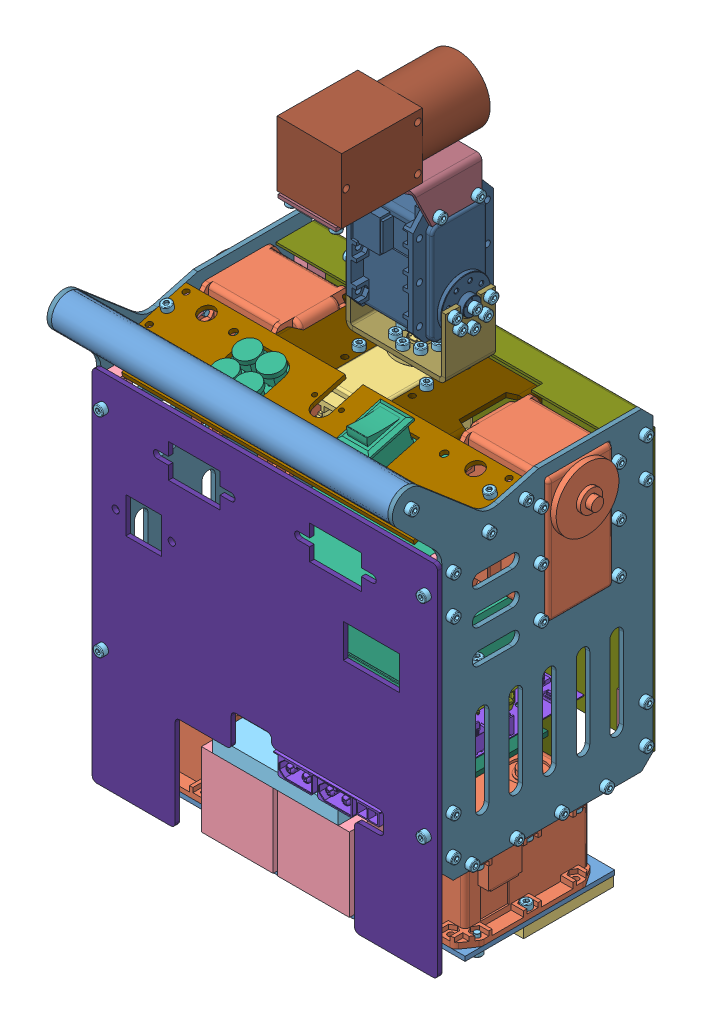
SolidWorks assembly 躯干, configuration 默认. Lengths in mm.
Overall size (172 287.24 163.85).
149 component instances, 24 part files, 310 mates.
Components (placement in the parent):
- 机器人-下腰骨-1: 机器人-下腰骨 [默认] at (14.1339 4.9855 143.3) size (150 2 94.2)
- 机器人-腰部连接件-1: 机器人-腰部连接件 [默认] at (86.3339 40.9855 146.55) size (5.6 6 68)
- 机器人-腰部连接件-2: 机器人-腰部连接件 [默认] at (-58.0661 40.9855 146.55) size (5.6 6 68)
- 机器人-腰部支撑件-1: 机器人-腰部支撑件 [默认] at (69.0339 0.6855 128.55) x (0 0 -1) z (1 0 0) size (40 4.3 40.2)
- 机器人-腰部支撑件-2: 机器人-腰部支撑件 [默认] at (-40.7661 0.6855 128.55) x (0 0 -1) z (1 0 0) size (40 4.3 40.2)
- 电池组-1: 电池组 [默认] at (-73.6661 8.3922 158.5613) x (0 -1 0) z (1 0 0) size (40 92 66)
  - 大电池-1: 大电池 [默认] at (-15.0933 -28.8887 72) size (33 78 32)
  - 大电池-2: 大电池 [默认] at (-15.0933 -28.8887 106) size (33 78 32)
  - 小电池-1: 小电池 [默认] at (-35.0933 63.1113 89) x (0 0 1) z (0 -1 0) size (56 7 92)
- 电路-1: 电路 [默认] at (-149.9254 121.6563 46.2423) x (0.629094 0.186421 -0.754644) z (0.775792 -0.211602 0.594451) size (135.66 81.1 136.29)
  - TX2-1: TX2 [默认] at (66.6739 -13.371 209.1651) x (-0.629094 -0.048866 -0.775792) z (0.186421 0.959412 -0.211602) size (87.07 50.04 32.13)
  - 9003-1: 9003 [默认] at (15.6894 -27.7493 144.427) x (0.629094 0.048866 0.775792) z (-0.186421 -0.959412 0.211602) size (96.22 72.67 50.58)
  - Main-1: Main [默认] at (20.5563 -29.3993 193.2183) x (0.629094 0.048866 0.775792) z (0.186421 0.959412 -0.211602) size (100 91.07 21.61)
- 机器人-背板-1: 机器人-背板 [默认] at (14.1339 173.2258 167.0875) x (1 0 0) z (0 -0.258819 0.965926) size (150 2 40)
- 脑袋-1: 脑袋 [默认] at (31.3694 207.3211 170.3695) x (-0.999965 0 -0.008321) z (0.008321 0 -0.999965) size (45.6 104.22 67.8)
  - MX28-2-1: MX28-2 [默认] at (67.0789 12.1977 37.204) x (0 0 -1) z (-1 0 0) size (35.6 50.71 44.45)
  - 工业摄像头-1: 工业摄像头 [默认] at (17.9784 61.4039 35.5741) x (-1 0 0) z (0 1 0) size (29 65.7 29)
  - 机器人-脖子-1: 机器人-脖子 [默认] at (17.6701 -26.3128 48.8741) size (106 27.37 22)
  - 机器人-摄像头固定件-1: 机器人-摄像头固定件 [默认] at (17.9784 46.9039 59.8741) x (-1 0 0) z (0 1 0) size (62.95 61 17.05)
- 机器人-侧板-3: 机器人-侧板 [默认] at (-60.8661 139.1722 141.05) x (0 0 1) z (-1 0 0) size (116.15 161.21 2)
- 机器人-侧板-4: 机器人-侧板 [默认] at (91.1339 139.1722 141.05) x (0 0 1) z (-1 0 0) size (116.15 161.21 2)
- 机器人-上腰骨-2: 机器人-上腰骨 [默认] at (14.1339 48.9855 149.05) size (100.8 2 61)
- 机器人-前盖-2: 机器人-前盖 [默认] at (14.1339 110.9855 94.95) x (1 0 0) z (0 -1 0) size (154 19.53 171.5)
- 机器人-后盖-2: 机器人-后盖 [默认] at (14.1339 100.9855 188.95) size (154 160 2)
- 机器人-肩骨-1: 机器人-肩骨 [默认] at (-24.8661 182.5355 128.55) size (28.68 11.38 40.2)
- 机器人-肩骨-2: 机器人-肩骨 [默认] at (53.1339 182.5355 128.55) x (-1 0 0) z (0 0 -1) size (28.68 11.38 40.2)
- 提手-1: 提手 [默认] at (-60.8661 194.6934 203.5985) size (150 15 15)
- MX64-1: MX64 [默认] at (69.0339 23.9855 128.55) x (-1 0 0) z (0 -1 0) size (40.2 62.1 50)
- MX64-2: MX64 [默认] at (-40.7661 23.9855 128.55) x (-1 0 0) z (0 -1 0) size (40.2 62.1 50)
- MX28-3: MX28 [默认] at (22.2109 109.2267 134.6509) x (1 0 0) z (0 1 0) size (35.6 50.71 42.85)
- MX64-3: MX64 [默认] at (-43.8661 162.8855 128.55) x (0 0 1) z (-1 0 0) size (40.2 62.1 50)
- MX64-4: MX64 [默认] at (72.1339 162.8855 128.55) x (0 0 -1) z (1 0 0) size (40.2 62.1 50)
- 机器人-盖子连接件-1: 机器人-盖子连接件 [默认] at (86.1339 152.4855 184.95) size (6 22 8)
- 机器人-盖子连接件-2: 机器人-盖子连接件 [默认] at (86.1339 59.4855 184.95) size (6 22 8)
- 机器人-盖子连接件-3: 机器人-盖子连接件 [默认] at (-57.8661 59.4855 184.95) size (6 22 8)
- 机器人-盖子连接件-4: 机器人-盖子连接件 [默认] at (-57.8661 152.4855 184.95) size (6 22 8)
- 机器人-盖子连接件-5: 机器人-盖子连接件 [默认] at (86.1339 162.4855 98.95) size (6 22 8)
- 机器人-盖子连接件-6: 机器人-盖子连接件 [默认] at (86.1339 59.4855 98.95) size (6 22 8)
- 机器人-盖子连接件-7: 机器人-盖子连接件 [默认] at (-57.8661 162.4855 98.95) size (6 22 8)
- 机器人-盖子连接件-8: 机器人-盖子连接件 [默认] at (-57.8661 59.4855 98.95) size (6 22 8)
- 机器人-盖子连接件-9: 机器人-盖子连接件 [默认] at (86.1339 170.7856 160.7396) x (1 0 0) z (0 0.965926 0.258819) size (6 22 8)
- 机器人-盖子连接件-10: 机器人-盖子连接件 [默认] at (-57.8661 170.7856 160.7396) x (1 0 0) z (0 0.965926 0.258819) size (6 22 8)
- hexagon socket head cap screws gb-5: hexagon socket head cap screws gb [GB_FASTENER_SCREWS_HSHCS M2.5X6-N] at (86.1339 59.4855 91.45) x (0 0 1) z (-1 0 0) size (8.5 4.5 4.5)
- hexagon socket head cap screws gb-6: hexagon socket head cap screws gb [GB_FASTENER_SCREWS_HSHCS M2.5X6-N] at (-57.8661 59.4855 91.45) x (0 0 1) z (-1 0 0) size (8.5 4.5 4.5)
- hexagon socket head cap screws gb-7: hexagon socket head cap screws gb [GB_FASTENER_SCREWS_HSHCS M2.5X6-N] at (86.1339 162.4855 91.45) x (0 0 1) z (-1 0 0) size (8.5 4.5 4.5)
- hexagon socket head cap screws gb-8: hexagon socket head cap screws gb [GB_FASTENER_SCREWS_HSHCS M2.5X6-N] at (-57.8661 162.4855 91.45) x (0 0 1) z (-1 0 0) size (8.5 4.5 4.5)
- hexagon socket head cap screws gb-9: hexagon socket head cap screws gb [GB_FASTENER_SCREWS_HSHCS M2.5X6-N] at (93.6339 170.9855 98.95) x (-1 0 0) z (0 0.924225 0.381849) size (8.5 4.5 4.5)
- hexagon socket head cap screws gb-10: hexagon socket head cap screws gb [GB_FASTENER_SCREWS_HSHCS M2.5X6-N] at (93.6339 153.9855 98.95) x (-1 0 0) z (0 0.924225 0.381849) size (8.5 4.5 4.5)
- hexagon socket head cap screws gb-11: hexagon socket head cap screws gb [GB_FASTENER_SCREWS_HSHCS M2.5X6-N] at (93.6339 67.9855 98.95) x (-1 0 0) z (0 0.924225 0.381849) size (8.5 4.5 4.5)
- hexagon socket head cap screws gb-12: hexagon socket head cap screws gb [GB_FASTENER_SCREWS_HSHCS M2.5X6-N] at (93.6339 50.9855 98.95) x (-1 0 0) z (0 0.924225 0.381849) size (8.5 4.5 4.5)
- hexagon socket head cap screws gb-13: hexagon socket head cap screws gb [GB_FASTENER_SCREWS_HSHCS M2.5X6-N] at (93.6339 43.9855 116.55) x (-1 0 0) z (0 0.924225 0.381849) size (8.5 4.5 4.5)
- hexagon socket head cap screws gb-14: hexagon socket head cap screws gb [GB_FASTENER_SCREWS_HSHCS M2.5X6-N] at (93.6339 43.9855 136.55) x (-1 0 0) z (0 0.924225 0.381849) size (8.5 4.5 4.5)
- hexagon socket head cap screws gb-15: hexagon socket head cap screws gb [GB_FASTENER_SCREWS_HSHCS M2.5X6-N] at (93.6339 43.9855 156.55) x (-1 0 0) z (0 0.924225 0.381849) size (8.5 4.5 4.5)
- hexagon socket head cap screws gb-16: hexagon socket head cap screws gb [GB_FASTENER_SCREWS_HSHCS M2.5X6-N] at (93.6339 43.9855 176.55) x (-1 0 0) z (0 0.924225 0.381849) size (8.5 4.5 4.5)
- hexagon socket head cap screws gb-17: hexagon socket head cap screws gb [GB_FASTENER_SCREWS_HSHCS M2.5X6-N] at (93.6339 50.9855 184.95) x (-1 0 0) z (0 0.924225 0.381849) size (8.5 4.5 4.5)
- hexagon socket head cap screws gb-18: hexagon socket head cap screws gb [GB_FASTENER_SCREWS_HSHCS M2.5X6-N] at (93.6339 67.9855 184.95) x (-1 0 0) z (0 0.924225 0.381849) size (8.5 4.5 4.5)
- hexagon socket head cap screws gb-19: hexagon socket head cap screws gb [GB_FASTENER_SCREWS_HSHCS M2.5X6-N] at (93.6339 160.9855 184.95) x (-1 0 0) z (0 0.924225 0.381849) size (8.5 4.5 4.5)
- hexagon socket head cap screws gb-20: hexagon socket head cap screws gb [GB_FASTENER_SCREWS_HSHCS M2.5X6-N] at (93.6339 143.9855 184.95) x (-1 0 0) z (0 0.924225 0.381849) size (8.5 4.5 4.5)
- hexagon socket head cap screws gb-21: hexagon socket head cap screws gb [GB_FASTENER_SCREWS_HSHCS M2.5X6-N] at (93.6339 168.5856 168.95) x (-1 0 0) z (0 0.924225 0.381849) size (8.5 4.5 4.5)
- hexagon socket head cap screws gb-22: hexagon socket head cap screws gb [GB_FASTENER_SCREWS_HSHCS M2.5X6-N] at (93.6339 172.9855 152.5293) x (-1 0 0) z (0 0.924225 0.381849) size (8.5 4.5 4.5)
- hexagon socket head cap screws gb-23: hexagon socket head cap screws gb [GB_FASTENER_SCREWS_HSHCS M2.5X6-N] at (-65.3661 170.9855 98.95) size (8.5 4.5 4.5)
- hexagon socket head cap screws gb-24: hexagon socket head cap screws gb [GB_FASTENER_SCREWS_HSHCS M2.5X6-N] at (-65.3661 153.9855 98.95) size (8.5 4.5 4.5)
- hexagon socket head cap screws gb-25: hexagon socket head cap screws gb [GB_FASTENER_SCREWS_HSHCS M2.5X6-N] at (-65.3661 67.9855 98.95) size (8.5 4.5 4.5)
- hexagon socket head cap screws gb-26: hexagon socket head cap screws gb [GB_FASTENER_SCREWS_HSHCS M2.5X6-N] at (-65.3661 50.9855 98.95) size (8.5 4.5 4.5)
- hexagon socket head cap screws gb-27: hexagon socket head cap screws gb [GB_FASTENER_SCREWS_HSHCS M2.5X6-N] at (-65.3661 43.9855 116.55) size (8.5 4.5 4.5)
- hexagon socket head cap screws gb-28: hexagon socket head cap screws gb [GB_FASTENER_SCREWS_HSHCS M2.5X6-N] at (-65.3661 43.9855 136.55) size (8.5 4.5 4.5)
- hexagon socket head cap screws gb-29: hexagon socket head cap screws gb [GB_FASTENER_SCREWS_HSHCS M2.5X6-N] at (-65.3661 43.9855 156.55) size (8.5 4.5 4.5)
- hexagon socket head cap screws gb-30: hexagon socket head cap screws gb [GB_FASTENER_SCREWS_HSHCS M2.5X6-N] at (-65.3661 43.9855 176.55) size (8.5 4.5 4.5)
- hexagon socket head cap screws gb-31: hexagon socket head cap screws gb [GB_FASTENER_SCREWS_HSHCS M2.5X6-N] at (-65.3661 50.9855 184.95) size (8.5 4.5 4.5)
- hexagon socket head cap screws gb-32: hexagon socket head cap screws gb [GB_FASTENER_SCREWS_HSHCS M2.5X6-N] at (-65.3661 67.9855 184.95) size (8.5 4.5 4.5)
- hexagon socket head cap screws gb-33: hexagon socket head cap screws gb [GB_FASTENER_SCREWS_HSHCS M2.5X6-N] at (-65.3661 143.9855 184.95) size (8.5 4.5 4.5)
- hexagon socket head cap screws gb-34: hexagon socket head cap screws gb [GB_FASTENER_SCREWS_HSHCS M2.5X6-N] at (-65.3661 160.9855 184.95) size (8.5 4.5 4.5)
- hexagon socket head cap screws gb-35: hexagon socket head cap screws gb [GB_FASTENER_SCREWS_HSHCS M2.5X6-N] at (-65.3661 168.5856 168.95) size (8.5 4.5 4.5)
- hexagon socket head cap screws gb-36: hexagon socket head cap screws gb [GB_FASTENER_SCREWS_HSHCS M2.5X6-N] at (-65.3661 172.9855 152.5293) size (8.5 4.5 4.5)
- hexagon socket head cap screws gb-37: hexagon socket head cap screws gb [GB_FASTENER_SCREWS_HSHCS M2.5X6-N] at (-57.8661 178.9959 162.9396) x (0 -0.965926 -0.258819) z (0.258819 -0.25 0.933013) size (8.5 4.5 4.5)
- hexagon socket head cap screws gb-38: hexagon socket head cap screws gb [GB_FASTENER_SCREWS_HSHCS M2.5X6-N] at (86.1339 178.9959 162.9396) x (0 -0.965926 -0.258819) z (0.258819 -0.25 0.933013) size (8.5 4.5 4.5)
- hexagon socket head cap screws gb-41: hexagon socket head cap screws gb [GB_FASTENER_SCREWS_HSHCS M2.5X6-N] at (-57.8661 59.4855 193.45) x (0 0 -1) z (1 0 0) size (8.5 4.5 4.5)
- hexagon socket head cap screws gb-42: hexagon socket head cap screws gb [GB_FASTENER_SCREWS_HSHCS M2.5X6-N] at (86.1339 59.4855 193.45) x (0 0 -1) z (1 0 0) size (8.5 4.5 4.5)
- hexagon socket head cap screws gb-43: hexagon socket head cap screws gb [GB_FASTENER_SCREWS_HSHCS M2.5X6-N] at (86.1339 152.4855 193.45) x (0 0 -1) z (1 0 0) size (8.5 4.5 4.5)
- hexagon socket head cap screws gb-44: hexagon socket head cap screws gb [GB_FASTENER_SCREWS_HSHCS M2.5X6-N] at (-57.8661 152.4855 193.45) x (0 0 -1) z (1 0 0) size (8.5 4.5 4.5)
- hexagon socket head cap screws gb-45: hexagon socket head cap screws gb [GB_FASTENER_SCREWS_HSHCS M2.5X6-N] at (-65.3661 166.8855 111.25) size (8.5 4.5 4.5)
- hexagon socket head cap screws gb-46: hexagon socket head cap screws gb [GB_FASTENER_SCREWS_HSHCS M2.5X6-N] at (-65.3661 144.8855 111.25) size (8.5 4.5 4.5)
- hexagon socket head cap screws gb-47: hexagon socket head cap screws gb [GB_FASTENER_SCREWS_HSHCS M2.5X6-N] at (-65.3661 144.8855 145.85) size (8.5 4.5 4.5)
- hexagon socket head cap screws gb-48: hexagon socket head cap screws gb [GB_FASTENER_SCREWS_HSHCS M2.5X6-N] at (-65.3661 122.8855 111.25) size (8.5 4.5 4.5)
- hexagon socket head cap screws gb-49: hexagon socket head cap screws gb [GB_FASTENER_SCREWS_HSHCS M2.5X6-N] at (-65.3661 122.8855 145.85) size (8.5 4.5 4.5)
- hexagon socket head cap screws gb-50: hexagon socket head cap screws gb [GB_FASTENER_SCREWS_HSHCS M2.5X6-N] at (-65.3661 166.8855 145.85) size (8.5 4.5 4.5)
- hexagon socket head cap screws gb-51: hexagon socket head cap screws gb [GB_FASTENER_SCREWS_HSHCS M2.5X6-N] at (-5.1993 240.1809 112.6891) x (0.999965 0 0.008321) z (-0.008321 0 0.999965) size (8.5 4.5 4.5)
- hexagon socket head cap screws gb-52: hexagon socket head cap screws gb [GB_FASTENER_SCREWS_HSHCS M2.5X6-N] at (-5.3408 240.1809 129.6885) x (0.999965 0 0.008321) z (-0.008321 0 0.999965) size (8.5 4.5 4.5)
- hexagon socket head cap screws gb-53: hexagon socket head cap screws gb [GB_FASTENER_SCREWS_HSHCS M2.5X6-N] at (32.9374 240.1809 113.0064) x (-0.999965 0 -0.008321) z (0.008321 0 -0.999965) size (8.5 4.5 4.5)
- hexagon socket head cap screws gb-54: hexagon socket head cap screws gb [GB_FASTENER_SCREWS_HSHCS M2.5X6-N] at (32.7959 240.1809 130.0058) x (-0.999965 0 -0.008321) z (0.008321 0 -0.999965) size (8.5 4.5 4.5)
- hexagon socket head cap screws gb-55: hexagon socket head cap screws gb [GB_FASTENER_SCREWS_HSHCS M2.5X6-N] at (93.6339 166.8855 145.85) x (-1 0 0) z (0 0.924225 0.381849) size (8.5 4.5 4.5)
- hexagon socket head cap screws gb-56: hexagon socket head cap screws gb [GB_FASTENER_SCREWS_HSHCS M2.5X6-N] at (93.6339 144.8855 145.85) x (-1 0 0) z (0 0.924225 0.381849) size (8.5 4.5 4.5)
- hexagon socket head cap screws gb-57: hexagon socket head cap screws gb [GB_FASTENER_SCREWS_HSHCS M2.5X6-N] at (93.6339 122.8855 145.85) x (-1 0 0) z (0 0.924225 0.381849) size (8.5 4.5 4.5)
- hexagon socket head cap screws gb-58: hexagon socket head cap screws gb [GB_FASTENER_SCREWS_HSHCS M2.5X6-N] at (93.6339 166.8855 111.25) x (-1 0 0) z (0 0.924225 0.381849) size (8.5 4.5 4.5)
- hexagon socket head cap screws gb-59: hexagon socket head cap screws gb [GB_FASTENER_SCREWS_HSHCS M2.5X6-N] at (93.6339 144.8855 111.25) x (-1 0 0) z (0 0.924225 0.381849) size (8.5 4.5 4.5)
- hexagon socket head cap screws gb-60: hexagon socket head cap screws gb [GB_FASTENER_SCREWS_HSHCS M2.5X6-N] at (93.6339 122.8855 111.25) x (-1 0 0) z (0 0.924225 0.381849) size (8.5 4.5 4.5)
- hexagon socket head cap screws gb-62: hexagon socket head cap screws gb [GB_FASTENER_SCREWS_HSHCS M2.5X6-N] at (38.9118 204.3809 129.5567) x (-0.999965 0 -0.008321) z (0.008321 0 -0.999965) size (8.5 4.5 4.5)
- hexagon socket head cap screws gb-63: hexagon socket head cap screws gb [GB_FASTENER_SCREWS_HSHCS M2.5X6-N] at (38.9313 198.724 127.2136) x (-0.999965 0 -0.008321) z (0.008321 0 -0.999965) size (8.5 4.5 4.5)
- hexagon socket head cap screws gb-64: hexagon socket head cap screws gb [GB_FASTENER_SCREWS_HSHCS M2.5X6-N] at (38.9784 196.3809 121.557) x (-0.999965 0 -0.008321) z (0.008321 0 -0.999965) size (8.5 4.5 4.5)
- hexagon socket head cap screws gb-65: hexagon socket head cap screws gb [GB_FASTENER_SCREWS_HSHCS M2.5X6-N] at (39.0255 198.724 115.9003) x (-0.999965 0 -0.008321) z (0.008321 0 -0.999965) size (8.5 4.5 4.5)
- hexagon socket head cap screws gb-66: hexagon socket head cap screws gb [GB_FASTENER_SCREWS_HSHCS M2.5X6-N] at (39.045 204.3809 113.5572) x (-0.999965 0 -0.008321) z (0.008321 0 -0.999965) size (8.5 4.5 4.5)
- hexagon socket head cap screws gb-71: hexagon socket head cap screws gb [GB_FASTENER_SCREWS_HSHCS M2.5X6-N] at (-10.6987 204.3809 113.1433) x (0.999965 0 0.008321) z (-0.008321 0 0.999965) size (8.5 4.5 4.5)
- hexagon socket head cap screws gb-72: hexagon socket head cap screws gb [GB_FASTENER_SCREWS_HSHCS M2.5X6-N] at (-10.7182 198.724 115.4864) x (0.999965 0 0.008321) z (-0.008321 0 0.999965) size (8.5 4.5 4.5)
- hexagon socket head cap screws gb-73: hexagon socket head cap screws gb [GB_FASTENER_SCREWS_HSHCS M2.5X6-N] at (-10.7652 196.3809 121.143) x (0.999965 0 0.008321) z (-0.008321 0 0.999965) size (8.5 4.5 4.5)
- hexagon socket head cap screws gb-74: hexagon socket head cap screws gb [GB_FASTENER_SCREWS_HSHCS M2.5X6-N] at (-10.8123 198.724 126.7997) x (0.999965 0 0.008321) z (-0.008321 0 0.999965) size (8.5 4.5 4.5)
- hexagon socket head cap screws gb-75: hexagon socket head cap screws gb [GB_FASTENER_SCREWS_HSHCS M2.5X6-N] at (-10.8318 204.3809 129.1428) x (0.999965 0 0.008321) z (-0.008321 0 0.999965) size (8.5 4.5 4.5)
- hexagon socket head cap screws gb-78: hexagon socket head cap screws gb [GB_FASTENER_SCREWS_HSHCS M2.5X6-N] at (86.3339 35.9855 168.55) x (0 1 0) z (0 0 1) size (8.5 4.5 4.5)
- hexagon socket head cap screws gb-79: hexagon socket head cap screws gb [GB_FASTENER_SCREWS_HSHCS M2.5X6-N] at (86.3339 35.9855 146.55) x (0 1 0) z (0 0 1) size (8.5 4.5 4.5)
- hexagon socket head cap screws gb-80: hexagon socket head cap screws gb [GB_FASTENER_SCREWS_HSHCS M2.5X6-N] at (86.3339 35.9855 124.55) x (0 1 0) z (0 0 1) size (8.5 4.5 4.5)
- hexagon socket head cap screws gb-81: hexagon socket head cap screws gb [GB_FASTENER_SCREWS_HSHCS M2.5X6-N] at (-58.0661 35.9855 124.55) x (0 1 0) z (0 0 1) size (8.5 4.5 4.5)
- hexagon socket head cap screws gb-82: hexagon socket head cap screws gb [GB_FASTENER_SCREWS_HSHCS M2.5X6-N] at (-58.0661 35.9855 146.55) x (0 1 0) z (0 0 1) size (8.5 4.5 4.5)
- hexagon socket head cap screws gb-83: hexagon socket head cap screws gb [GB_FASTENER_SCREWS_HSHCS M2.5X6-N] at (-58.0661 35.9855 168.55) x (0 1 0) z (0 0 1) size (8.5 4.5 4.5)
- hexagon socket head cap screws gb-84: hexagon socket head cap screws gb [GB_FASTENER_SCREWS_HSHCS M2.5X6-N] at (-58.0661 11.9855 124.55) x (0 -1 0) z (0 0 1) size (8.5 4.5 4.5)
- hexagon socket head cap screws gb-85: hexagon socket head cap screws gb [GB_FASTENER_SCREWS_HSHCS M2.5X6-N] at (-58.0661 11.9855 146.55) x (0 -1 0) z (0 0 1) size (8.5 4.5 4.5)
- hexagon socket head cap screws gb-86: hexagon socket head cap screws gb [GB_FASTENER_SCREWS_HSHCS M2.5X6-N] at (-58.0661 2.4855 168.55) x (0 1 0) z (0 0 1) size (8.5 4.5 4.5)
- hexagon socket head cap screws gb-87: hexagon socket head cap screws gb [GB_FASTENER_SCREWS_HSHCS M2.5X6-N] at (-23.4661 2.4855 168.55) x (0 1 0) z (0 0 1) size (8.5 4.5 4.5)
- hexagon socket head cap screws gb-89: hexagon socket head cap screws gb [GB_FASTENER_SCREWS_HSHCS M2.5X6-N] at (86.3339 11.9855 146.55) x (0 -1 0) z (0 0 1) size (8.5 4.5 4.5)
- hexagon socket head cap screws gb-90: hexagon socket head cap screws gb [GB_FASTENER_SCREWS_HSHCS M2.5X6-N] at (86.3339 117.6114 168.55) x (0 -1 0) z (0 0 1) size (8.5 4.5 4.5)
- hexagon socket head cap screws gb-91: hexagon socket head cap screws gb [GB_FASTENER_SCREWS_HSHCS M2.5X6-N] at (86.3339 2.4855 168.55) x (0 1 0) z (0 0 1) size (8.5 4.5 4.5)
- hexagon socket head cap screws gb-92: hexagon socket head cap screws gb [GB_FASTENER_SCREWS_HSHCS M2.5X6-N] at (-23.4661 11.9855 124.55) x (0 -1 0) z (0 0 1) size (8.5 4.5 4.5)
- hexagon socket head cap screws gb-93: hexagon socket head cap screws gb [GB_FASTENER_SCREWS_HSHCS M2.5X6-N] at (-23.4661 11.9855 146.55) x (0 -1 0) z (0 0 1) size (8.5 4.5 4.5)
- hexagon socket head cap screws gb-94: hexagon socket head cap screws gb [GB_FASTENER_SCREWS_HSHCS M2.5X6-N] at (51.7339 11.9855 124.55) x (0 -1 0) z (0 0 1) size (8.5 4.5 4.5)
- hexagon socket head cap screws gb-95: hexagon socket head cap screws gb [GB_FASTENER_SCREWS_HSHCS M2.5X6-N] at (51.7339 11.9855 146.55) x (0 -1 0) z (0 0 1) size (8.5 4.5 4.5)
- hexagon socket head cap screws gb-96: hexagon socket head cap screws gb [GB_FASTENER_SCREWS_HSHCS M2.5X6-N] at (50.6339 166.8855 111.25) size (8.5 4.5 4.5)
- hexagon socket head cap screws gb-97: hexagon socket head cap screws gb [GB_FASTENER_SCREWS_HSHCS M2.5X6-N] at (29.1612 177.7582 116.85) x (0 -1 0) z (0 0 1) size (8.5 4.5 4.5)
- hexagon socket head cap screws gb-98: hexagon socket head cap screws gb [GB_FASTENER_SCREWS_HSHCS M2.5X6-N] at (-0.8934 177.7582 116.85) x (0 -1 0) z (0 0 1) size (8.5 4.5 4.5)
- hexagon socket head cap screws gb-99: hexagon socket head cap screws gb [GB_FASTENER_SCREWS_HSHCS M2.5X6-N] at (-22.3661 166.8855 111.25) x (-1 0 0) z (0 0.924225 0.381849) size (8.5 4.5 4.5)
- hexagon socket head cap screws gb-100: hexagon socket head cap screws gb [GB_FASTENER_SCREWS_HSHCS M2.5X6-N] at (14.1066 184.3582 121.35) x (0 -1 0) z (0 0 1) size (8.5 4.5 4.5)
- hexagon socket head cap screws gb-101: hexagon socket head cap screws gb [GB_FASTENER_SCREWS_HSHCS M2.5X6-N] at (39.8284 204.3809 121.564) x (-0.999965 0 -0.008321) z (0.008321 0 -0.999965) size (8.5 4.5 4.5)
- hexagon socket head cap screws gb-102: hexagon socket head cap screws gb [GB_FASTENER_SCREWS_HSHCS M2.5X6-N] at (-8.6199 204.3809 121.1609) x (0.999965 0 0.008321) z (-0.008321 0 0.999965) size (8.5 4.5 4.5)
- hexagon socket head cap screws gb-103: hexagon socket head cap screws gb [GB_FASTENER_SCREWS_HSHCS M2.5X6-N] at (-0.8934 177.7582 133.85) x (0 -1 0) z (0 0 1) size (8.5 4.5 4.5)
- hexagon socket head cap screws gb-104: hexagon socket head cap screws gb [GB_FASTENER_SCREWS_HSHCS M2.5X6-N] at (-22.3661 166.8855 145.85) x (-1 0 0) z (0 0.924225 0.381849) size (8.5 4.5 4.5)
- hexagon socket head cap screws gb-105: hexagon socket head cap screws gb [GB_FASTENER_SCREWS_HSHCS M2.5X6-N] at (50.6339 166.8855 145.85) size (8.5 4.5 4.5)
- hexagon socket head cap screws gb-106: hexagon socket head cap screws gb [GB_FASTENER_SCREWS_HSHCS M2.5X6-N] at (29.1612 177.7582 133.85) x (0 -1 0) z (0 0 1) size (8.5 4.5 4.5)
- hexagon socket head cap screws gb-107: hexagon socket head cap screws gb [GB_FASTENER_SCREWS_HSHCS M2.5X6-N] at (8.497 183.5082 115.6463) x (0 -1 0) z (0 0 1) size (8.5 4.5 4.5)
- hexagon socket head cap screws gb-108: hexagon socket head cap screws gb [GB_FASTENER_SCREWS_HSHCS M2.5X6-N] at (6.1069 183.5082 121.2834) x (0 -1 0) z (0 0 1) size (8.5 4.5 4.5)
- hexagon socket head cap screws gb-109: hexagon socket head cap screws gb [GB_FASTENER_SCREWS_HSHCS M2.5X6-N] at (8.4029 183.5082 126.9596) x (0 -1 0) z (0 0 1) size (8.5 4.5 4.5)
- hexagon socket head cap screws gb-110: hexagon socket head cap screws gb [GB_FASTENER_SCREWS_HSHCS M2.5X6-N] at (14.04 183.5082 129.3497) x (0 -1 0) z (0 0 1) size (8.5 4.5 4.5)
- hexagon socket head cap screws gb-111: hexagon socket head cap screws gb [GB_FASTENER_SCREWS_HSHCS M2.5X6-N] at (19.7162 183.5082 127.0537) x (0 -1 0) z (0 0 1) size (8.5 4.5 4.5)
- hexagon socket head cap screws gb-112: hexagon socket head cap screws gb [GB_FASTENER_SCREWS_HSHCS M2.5X6-N] at (22.1063 183.5082 121.4166) x (0 -1 0) z (0 0 1) size (8.5 4.5 4.5)
- hexagon socket head cap screws gb-113: hexagon socket head cap screws gb [GB_FASTENER_SCREWS_HSHCS M2.5X6-N] at (19.8103 183.5082 115.7404) x (0 -1 0) z (0 0 1) size (8.5 4.5 4.5)
- hexagon socket head cap screws gb-114: hexagon socket head cap screws gb [GB_FASTENER_SCREWS_HSHCS M2.5X6-N] at (14.1732 183.5082 113.3503) x (0 -1 0) z (0 0 1) size (8.5 4.5 4.5)
- hexagon socket head cap screws gb-115: hexagon socket head cap screws gb [GB_FASTENER_SCREWS_HSHCS M2.5X6-N] at (93.6339 194.6934 203.5985) x (-1 0 0) z (0 0.924225 0.381849) size (8.5 4.5 4.5)
- hexagon socket head cap screws gb-116: hexagon socket head cap screws gb [GB_FASTENER_SCREWS_HSHCS M2.5X6-N] at (-65.3661 194.6934 203.5985) size (8.5 4.5 4.5)
- hexagon socket head cap screws gb-117: hexagon socket head cap screws gb [GB_FASTENER_SCREWS_HSHCS M2.5X6-N] at (23.6707 250.2249 136.7301) x (0 1 0) z (-0.004657 0 0.999989) size (8.5 4.5 4.5)
- hexagon socket head cap screws gb-118: hexagon socket head cap screws gb [GB_FASTENER_SCREWS_HSHCS M2.5X6-N] at (3.6713 250.2249 136.5637) x (0 1 0) z (-0.004657 0 0.999989) size (8.5 4.5 4.5)
- hexagon socket head cap screws gb-119: hexagon socket head cap screws gb [GB_FASTENER_SCREWS_HSHCS M2.5X6-N] at (3.4076 250.2249 168.2626) x (0 1 0) z (-0.004657 0 0.999989) size (8.5 4.5 4.5)
- hexagon socket head cap screws gb-120: hexagon socket head cap screws gb [GB_FASTENER_SCREWS_HSHCS M2.5X6-N] at (23.4069 250.2249 168.429) x (0 1 0) z (-0.004657 0 0.999989) size (8.5 4.5 4.5)
- Back-1: Back [默认] at (14.1339 170.328 166.311) x (1 0 0) z (0 0.965926 0.258819) size (100 30 26.32)
Mates (geometry in assembly coordinates):
- 同心1: concentric: cylinder of assembly; cylinder of assembly; cylinder of 机器人-下腰骨-1 through (-58.0661 6.9855 124.55) axis (0 -1 0) radius 1.35; cylinder of MX64-2 through (-58.0661 6.9855 124.55) axis (0 1 0) radius 1.35
- 同心2: concentric: cylinder of assembly; cylinder of assembly; cylinder of 机器人-下腰骨-1 through (-58.0661 6.9855 146.55) axis (0 -1 0) radius 1.35; cylinder of MX64-2 through (-58.0661 6.9855 146.55) axis (0 1 0) radius 1.35
- 重合1: coincident: plane of assembly; plane of assembly; plane of 机器人-下腰骨-1 through (14.1339 6.9855 143.3) normal (0 1 0); plane of MX64-2 through (-19.8621 6.9855 177.872) normal (0 -1 0)
- 同心3: concentric: cylinder of assembly; cylinder of assembly; cylinder of 机器人-下腰骨-1 through (86.3339 6.9855 124.55) axis (0 -1 0) radius 1.35; cylinder of MX64-1 through (86.3339 6.9855 124.55) axis (0 1 0) radius 1.35
- 同心4: concentric: cylinder of assembly; cylinder of assembly; cylinder of 机器人-下腰骨-1 through (86.3339 6.9855 146.55) axis (0 -1 0) radius 1.35; cylinder of MX64-1 through (86.3339 6.9855 146.55) axis (0 1 0) radius 1.35
- 重合2: coincident: plane of assembly; plane of assembly; plane of 机器人-下腰骨-1 through (14.1339 6.9855 143.3) normal (0 1 0); plane of MX64-1 through (89.9379 6.9855 177.872) normal (0 -1 0)
- 同心11: concentric: cylinder of assembly; cylinder of assembly; cylinder of MX64-2 through (-58.0661 38.4855 168.55) axis (0 1 0) radius 1.35; cylinder of 机器人-腰部连接件-2 through (-58.0661 46.9865 168.55) axis (0 -1 0) radius 1
- 同心12: concentric: cylinder of assembly; cylinder of assembly; cylinder of MX64-2 through (-58.0661 38.4855 124.55) axis (0 1 0) radius 1.35; cylinder of 机器人-腰部连接件-2 through (-58.0661 46.9865 124.55) axis (0 -1 0) radius 1
- 重合6: coincident: plane of assembly; plane of assembly; plane of MX64-2 through (-19.8621 40.9855 177.872) normal (0 1 0); plane of 机器人-腰部连接件-2 through (-55.2661 40.9855 180.55) normal (0 -1 0)
- 同心14: concentric: cylinder of assembly; cylinder of assembly; cylinder of MX64-1 through (86.3339 38.4855 168.55) axis (0 1 0) radius 1.35; cylinder of 机器人-腰部连接件-1 through (86.3339 46.9865 168.55) axis (0 -1 0) radius 1
- 同心15: concentric: cylinder of assembly; cylinder of assembly; cylinder of MX64-1 through (86.3339 38.4855 124.55) axis (0 1 0) radius 1.35; cylinder of 机器人-腰部连接件-1 through (86.3339 46.9865 124.55) axis (0 -1 0) radius 1
- 重合7: coincident: plane of assembly; plane of assembly; plane of MX64-1 through (89.9379 40.9855 177.872) normal (0 1 0); plane of 机器人-腰部连接件-1 through (89.1339 40.9855 180.55) normal (0 -1 0)
- 同心36: concentric: cylinder of assembly; cylinder of assembly; cylinder of MX64-1 through (69.0339 0.4855 128.55) axis (0 1 0) radius 14; cylinder of 机器人-腰部支撑件-1 through (69.0339 3.1855 128.55) axis (0 -1 0) radius 14.3
- 同心37: concentric: cylinder of assembly; cylinder of assembly; cylinder of 机器人-下腰骨-1 through (86.3339 6.9855 124.55) axis (0 -1 0) radius 1.35; cylinder of 机器人-腰部支撑件-1 through (86.3339 0.6845 124.55) axis (0 1 0) radius 1
- 重合20: coincident: plane of assembly; plane of assembly; plane of 机器人-下腰骨-1 through (14.1339 4.9855 143.3) normal (0 -1 0); plane of 机器人-腰部支撑件-1 through (69.0339 4.9855 128.55) normal (0 1 0)
- 同心38: concentric: cylinder of assembly; cylinder of assembly; cylinder of MX64-2 through (-40.7661 0.4855 128.55) axis (0 1 0) radius 14; cylinder of 机器人-腰部支撑件-2 through (-40.7661 3.1855 128.55) axis (0 -1 0) radius 14.3
- 同心39: concentric: cylinder of assembly; cylinder of assembly; cylinder of MX64-2 through (-23.4661 6.9855 124.55) axis (0 1 0) radius 1.35; cylinder of 机器人-腰部支撑件-2 through (-23.4661 0.6845 124.55) axis (0 1 0) radius 1
- 重合21: coincident: plane of assembly; plane of assembly; plane of 机器人-下腰骨-1 through (14.1339 4.9855 143.3) normal (0 -1 0); plane of 机器人-腰部支撑件-2 through (-40.7661 4.9855 128.55) normal (0 1 0)
- 同心151: concentric: cylinder of MX28-3 through (14.1066 181.6741 121.35) axis (0 -1 0) radius 4; cylinder of ? through (14.1066 181.5082 121.35) axis (0 -1 0) radius 4.5
- 重合88: coincident: plane of MX28-3 through (23.8638 179.0082 133.8914) normal (0 1 0); plane of ? through (14.1066 179.0082 121.35) normal (0 -1 0)
- 同心152: concentric: cylinder of assembly; cylinder of assembly; cylinder of MX64-3 through (-60.8661 166.8855 111.25) axis (1 0 0) radius 1.35; cylinder of 机器人-侧板-3 through (-62.8661 166.8855 111.25) axis (1 0 0) radius 1.35
- 同心153: concentric: cylinder of assembly; cylinder of assembly; cylinder of MX64-3 through (-60.8661 144.8855 111.25) axis (1 0 0) radius 1.35; cylinder of 机器人-侧板-3 through (-62.8661 144.8855 111.25) axis (1 0 0) radius 1.35
- 重合89: coincident: plane of assembly; plane of assembly; plane of MX64-3 through (-60.8661 113.5635 107.646) normal (-1 0 0); plane of 机器人-侧板-3 through (-60.8661 139.1722 141.05) normal (1 0 0)
- 同心154: concentric: cylinder of assembly; cylinder of assembly; cylinder of 机器人-腰部连接件-2 through (-60.8671 43.9855 116.55) axis (1 0 0) radius 1; cylinder of 机器人-侧板-3 through (-62.8661 43.9855 116.55) axis (1 0 0) radius 1.35
- 同心155: concentric: cylinder of assembly; cylinder of assembly; cylinder of 机器人-腰部连接件-2 through (-60.8671 43.9855 136.55) axis (1 0 0) radius 1; cylinder of 机器人-侧板-3 through (-62.8661 43.9855 136.55) axis (1 0 0) radius 1.35
- 重合90: coincident: plane of assembly; plane of assembly; plane of 机器人-腰部连接件-2 through (-60.8661 40.9855 180.55) normal (-1 0 0); plane of 机器人-侧板-3 through (-60.8661 139.1722 141.05) normal (1 0 0)
- 同心156: concentric: cylinder of assembly; cylinder of assembly; cylinder of MX64-4 through (89.1339 166.8855 145.85) axis (-1 0 0) radius 1.35; cylinder of 机器人-侧板-4 through (89.1339 166.8855 145.85) axis (1 0 0) radius 1.35
- 同心157: concentric: cylinder of assembly; cylinder of assembly; cylinder of MX64-4 through (89.1339 144.8855 145.85) axis (-1 0 0) radius 1.35; cylinder of 机器人-侧板-4 through (89.1339 144.8855 145.85) axis (1 0 0) radius 1.35
- 重合91: coincident: plane of assembly; plane of assembly; plane of MX64-4 through (89.1339 113.5635 149.454) normal (1 0 0); plane of 机器人-侧板-4 through (89.1339 139.1722 141.05) normal (-1 0 0)
- 同心158: concentric: cylinder of assembly; cylinder of assembly; cylinder of 机器人-腰部连接件-1 through (83.5329 43.9855 116.55) axis (1 0 0) radius 1; cylinder of 机器人-侧板-4 through (89.1339 43.9855 116.55) axis (1 0 0) radius 1.35
- 同心159: concentric: cylinder of assembly; cylinder of assembly; cylinder of 机器人-腰部连接件-1 through (83.5329 43.9855 136.55) axis (1 0 0) radius 1; cylinder of 机器人-侧板-4 through (89.1339 43.9855 136.55) axis (1 0 0) radius 1.35
- 重合92: coincident: plane of assembly; plane of assembly; plane of 机器人-腰部连接件-1 through (89.1339 46.9855 180.55) normal (1 0 0); plane of 机器人-侧板-4 through (89.1339 139.1722 141.05) normal (-1 0 0)
- 同心167: concentric: cylinder of ? through (-33.8661 49.4845 117.55) axis (0 1 0) radius 1.6; cylinder of 机器人-上腰骨-2 through (-33.8661 50.9855 117.55) axis (0 -1 0) radius 1.6
- 同心168: concentric: cylinder of ? through (-33.8661 49.4845 157.55) axis (0 1 0) radius 1.6; cylinder of 机器人-上腰骨-2 through (-33.8661 50.9855 157.55) axis (0 -1 0) radius 1.6
- 距离11: distance = 7 mm: plane of ? through (14.1339 57.9855 137.55) normal (0 -1 0); plane of 机器人-上腰骨-2 through (14.1339 50.9855 149.05) normal (0 1 0)
- 同心169: concentric: cylinder of assembly; cylinder of assembly; cylinder of MX64-2 through (-29.7661 38.4855 173.85) axis (0 1 0) radius 1.35; cylinder of 机器人-上腰骨-2 through (-29.7661 50.9855 173.85) axis (0 -1 0) radius 1.35
- 同心170: concentric: cylinder of assembly; cylinder of assembly; cylinder of MX64-2 through (-23.4661 38.4855 124.55) axis (0 1 0) radius 1.35; cylinder of 机器人-上腰骨-2 through (-23.4661 50.9855 124.55) axis (0 -1 0) radius 1.35
- 距离12: distance = 8 mm: plane of assembly; plane of assembly; plane of 机器人-上腰骨-2 through (14.1339 48.9855 149.05) normal (0 -1 0); plane of MX64-2 through (-19.8621 40.9855 177.872) normal (0 1 0)
- 同心193: concentric: cylinder of assembly; cylinder of assembly; cylinder of MX64-3 through (-29.3661 166.8855 145.85) axis (1 0 0) radius 1.35; cylinder of 机器人-肩骨-1 through (-26.8661 166.8855 145.85) axis (1 0 0) radius 1.35
- 同心194: concentric: cylinder of assembly; cylinder of assembly; cylinder of MX64-3 through (-29.3661 166.8855 111.25) axis (1 0 0) radius 1.35; cylinder of 机器人-肩骨-1 through (-26.8661 166.8855 111.25) axis (1 0 0) radius 1.35
- 重合108: coincident: plane of assembly; plane of assembly; plane of MX64-3 through (-26.8661 113.5635 107.646) normal (1 0 0); plane of 机器人-肩骨-1 through (-26.8661 182.5355 128.55) normal (-1 0 0)
- 同心195: concentric: cylinder of assembly; cylinder of assembly; cylinder of MX64-4 through (57.6339 166.8855 111.25) axis (-1 0 0) radius 1.35; cylinder of 机器人-肩骨-2 through (55.1339 166.8855 111.25) axis (-1 0 0) radius 1.35
- 同心196: concentric: cylinder of assembly; cylinder of assembly; cylinder of MX64-4 through (57.6339 166.8855 145.85) axis (-1 0 0) radius 1.35; cylinder of 机器人-肩骨-2 through (55.1339 166.8855 145.85) axis (-1 0 0) radius 1.35
- 重合109: coincident: plane of assembly; plane of assembly; plane of MX64-4 through (55.1339 113.5635 149.454) normal (-1 0 0); plane of 机器人-肩骨-2 through (55.1339 182.5355 128.55) normal (1 0 0)
- 同心197: concentric: cylinder of assembly; cylinder of assembly; cylinder of MX28-3 through (-0.8934 173.2582 116.85) axis (0 -1 0) radius 1.35; cylinder of 机器人-肩骨-1 through (-0.8934 175.2582 116.85) axis (0 -1 0) radius 1.35
- 同心198: concentric: cylinder of assembly; cylinder of assembly; cylinder of MX28-3 through (-0.8934 173.2582 133.85) axis (0 -1 0) radius 1.35; cylinder of 机器人-肩骨-1 through (-0.8934 175.2582 133.85) axis (0 -1 0) radius 1.35
- 重合110: coincident: plane of assembly; plane of assembly; plane of MX28-3 through (-4.4054 173.2582 160.962) normal (0 1 0); plane of 机器人-肩骨-1 through (-16.8434 173.2582 128.55) normal (0 -1 0)
- 同心199: concentric: cylinder of assembly; cylinder of assembly; cylinder of 机器人-侧板-4 through (91.1339 194.6934 203.5985) axis (-1 0 0) radius 1.6; cylinder of 提手-1 through (89.1339 194.6934 203.5985) axis (-1 0 0) radius 7.5
- 同心200: concentric: cylinder of assembly; cylinder of assembly; cylinder of MX28-3 through (14.1066 181.6741 121.35) axis (0 -1 0) radius 4; cylinder of 脑袋-1/机器人-脖子-1 through (14.1066 179.0082 121.35) axis (0 1 0) radius 4.5
- 重合112: coincident: plane of assembly; plane of assembly; plane of MX28-3 through (23.8638 179.0082 133.8914) normal (0 1 0); plane of 脑袋-1/机器人-脖子-1 through (59.105 179.0082 121.7244) normal (0 -1 0)
- 重合113: coincident: plane of assembly; plane of assembly; plane of 机器人-侧板-4 through (89.1339 139.1722 141.05) normal (-1 0 0); plane of 提手-1 through (89.1339 194.6934 203.5985) normal (1 0 0)
- 同心201: concentric: cylinder of assembly; cylinder of assembly; cylinder of 机器人-侧板-3 through (-60.8651 170.9855 98.95) axis (-1 0 0) radius 1.35; cylinder of 机器人-盖子连接件-7 through (-54.8661 170.9855 98.95) axis (-1 0 0) radius 1.25
- 同心202: concentric: cylinder of assembly; cylinder of assembly; cylinder of 机器人-侧板-3 through (-60.8651 153.9855 98.95) axis (-1 0 0) radius 1.35; cylinder of 机器人-盖子连接件-7 through (-54.8661 153.9855 98.95) axis (-1 0 0) radius 1.25
- 重合116: coincident: plane of assembly; plane of assembly; plane of 机器人-侧板-3 through (-60.8661 139.1722 141.05) normal (1 0 0); plane of 机器人-盖子连接件-7 through (-60.8661 173.4855 94.95) normal (-1 0 0)
- 同心203: concentric: cylinder of assembly; cylinder of assembly; cylinder of 机器人-侧板-3 through (-60.8651 67.9855 98.95) axis (-1 0 0) radius 1.35; cylinder of 机器人-盖子连接件-8 through (-54.8661 67.9855 98.95) axis (-1 0 0) radius 1.25
- 同心204: concentric: cylinder of assembly; cylinder of assembly; cylinder of 机器人-侧板-3 through (-60.8651 50.9855 98.95) axis (-1 0 0) radius 1.35; cylinder of 机器人-盖子连接件-8 through (-54.8661 50.9855 98.95) axis (-1 0 0) radius 1.25
- 重合118: coincident: plane of assembly; plane of assembly; plane of 机器人-侧板-3 through (-60.8661 139.1722 141.05) normal (1 0 0); plane of 机器人-盖子连接件-8 through (-60.8661 70.4855 94.95) normal (-1 0 0)
- 同心205: concentric: cylinder of assembly; cylinder of assembly; cylinder of 机器人-侧板-4 through (91.1349 67.9855 98.95) axis (-1 0 0) radius 1.35; cylinder of 机器人-盖子连接件-6 through (89.1339 67.9855 98.95) axis (-1 0 0) radius 1.25
- 同心206: concentric: cylinder of assembly; cylinder of assembly; cylinder of 机器人-侧板-4 through (91.1349 50.9855 98.95) axis (-1 0 0) radius 1.35; cylinder of 机器人-盖子连接件-6 through (89.1339 50.9855 98.95) axis (-1 0 0) radius 1.25
- 重合119: coincident: plane of assembly; plane of assembly; plane of 机器人-侧板-4 through (89.1339 139.1722 141.05) normal (-1 0 0); plane of 机器人-盖子连接件-6 through (89.1339 70.4855 94.95) normal (1 0 0)
- 同心207: concentric: cylinder of assembly; cylinder of assembly; cylinder of 机器人-侧板-4 through (91.1349 170.9855 98.95) axis (-1 0 0) radius 1.35; cylinder of 机器人-盖子连接件-5 through (89.1339 170.9855 98.95) axis (-1 0 0) radius 1.25
- 同心208: concentric: cylinder of assembly; cylinder of assembly; cylinder of 机器人-侧板-4 through (91.1349 153.9855 98.95) axis (-1 0 0) radius 1.35; cylinder of 机器人-盖子连接件-5 through (89.1339 153.9855 98.95) axis (-1 0 0) radius 1.25
- 重合120: coincident: plane of assembly; plane of assembly; plane of 机器人-侧板-4 through (89.1339 139.1722 141.05) normal (-1 0 0); plane of 机器人-盖子连接件-5 through (89.1339 173.4855 94.95) normal (1 0 0)
- 同心209: concentric: cylinder of assembly; cylinder of assembly; cylinder of 机器人-侧板-4 through (91.1349 160.9855 184.95) axis (-1 0 0) radius 1.35; cylinder of 机器人-盖子连接件-1 through (89.1339 160.9855 184.95) axis (-1 0 0) radius 1.25
- 同心210: concentric: cylinder of assembly; cylinder of assembly; cylinder of 机器人-侧板-4 through (91.1349 143.9855 184.95) axis (-1 0 0) radius 1.35; cylinder of 机器人-盖子连接件-1 through (89.1339 143.9855 184.95) axis (-1 0 0) radius 1.25
- 重合121: coincident: plane of assembly; plane of assembly; plane of 机器人-侧板-4 through (89.1339 139.1722 141.05) normal (-1 0 0); plane of 机器人-盖子连接件-1 through (89.1339 163.4855 180.95) normal (1 0 0)
- 同心211: concentric: cylinder of assembly; cylinder of assembly; cylinder of 机器人-侧板-4 through (91.1349 67.9855 184.95) axis (-1 0 0) radius 1.35; cylinder of 机器人-盖子连接件-2 through (89.1339 67.9855 184.95) axis (-1 0 0) radius 1.25
- 同心212: concentric: cylinder of assembly; cylinder of assembly; cylinder of 机器人-侧板-4 through (91.1349 50.9855 184.95) axis (-1 0 0) radius 1.35; cylinder of 机器人-盖子连接件-2 through (89.1339 50.9855 184.95) axis (-1 0 0) radius 1.25
- 重合122: coincident: plane of assembly; plane of assembly; plane of 机器人-侧板-4 through (89.1339 139.1722 141.05) normal (-1 0 0); plane of 机器人-盖子连接件-2 through (89.1339 70.4855 180.95) normal (1 0 0)
- 同心213: concentric: cylinder of assembly; cylinder of assembly; cylinder of 机器人-侧板-3 through (-60.8651 67.9855 184.95) axis (-1 0 0) radius 1.35; cylinder of 机器人-盖子连接件-3 through (-54.8661 67.9855 184.95) axis (-1 0 0) radius 1.25
- 同心214: concentric: cylinder of assembly; cylinder of assembly; cylinder of 机器人-侧板-3 through (-60.8651 50.9855 184.95) axis (-1 0 0) radius 1.35; cylinder of 机器人-盖子连接件-3 through (-54.8661 50.9855 184.95) axis (-1 0 0) radius 1.25
- 重合123: coincident: plane of assembly; plane of assembly; plane of 机器人-侧板-3 through (-60.8661 139.1722 141.05) normal (1 0 0); plane of 机器人-盖子连接件-3 through (-60.8661 70.4855 180.95) normal (-1 0 0)
- 同心215: concentric: cylinder of assembly; cylinder of assembly; cylinder of 机器人-侧板-3 through (-60.8651 160.9855 184.95) axis (-1 0 0) radius 1.35; cylinder of 机器人-盖子连接件-4 through (-54.8661 160.9855 184.95) axis (-1 0 0) radius 1.25
- 同心216: concentric: cylinder of assembly; cylinder of assembly; cylinder of 机器人-侧板-3 through (-60.8651 143.9855 184.95) axis (-1 0 0) radius 1.35; cylinder of 机器人-盖子连接件-4 through (-54.8661 143.9855 184.95) axis (-1 0 0) radius 1.25
- 重合124: coincident: plane of assembly; plane of assembly; plane of 机器人-侧板-3 through (-60.8661 139.1722 141.05) normal (1 0 0); plane of 机器人-盖子连接件-4 through (-60.8661 163.4855 180.95) normal (-1 0 0)
- 同心217: concentric: cylinder of assembly; cylinder of assembly; cylinder of 机器人-侧板-3 through (-60.8651 168.5856 168.95) axis (-1 0 0) radius 1.35; cylinder of 机器人-盖子连接件-10 through (-54.8661 168.5856 168.95) axis (-1 0 0) radius 1.25
- 同心218: concentric: cylinder of assembly; cylinder of assembly; cylinder of 机器人-侧板-3 through (-60.8651 172.9855 152.5293) axis (-1 0 0) radius 1.35; cylinder of 机器人-盖子连接件-10 through (-54.8661 172.9855 152.5293) axis (-1 0 0) radius 1.25
- 重合125: coincident: plane of assembly; plane of assembly; plane of 机器人-侧板-3 through (-60.8661 139.1722 141.05) normal (1 0 0); plane of 机器人-盖子连接件-10 through (-60.8661 169.7689 149.0792) normal (-1 0 0)
- 同心219: concentric: cylinder of assembly; cylinder of assembly; cylinder of 机器人-侧板-4 through (91.1349 168.5856 168.95) axis (-1 0 0) radius 1.35; cylinder of 机器人-盖子连接件-9 through (89.1339 168.5856 168.95) axis (-1 0 0) radius 1.25
- 同心220: concentric: cylinder of assembly; cylinder of assembly; cylinder of 机器人-侧板-4 through (91.1349 172.9855 152.5293) axis (-1 0 0) radius 1.35; cylinder of 机器人-盖子连接件-9 through (89.1339 172.9855 152.5293) axis (-1 0 0) radius 1.25
- 重合126: coincident: plane of assembly; plane of assembly; plane of 机器人-侧板-4 through (89.1339 139.1722 141.05) normal (-1 0 0); plane of 机器人-盖子连接件-9 through (89.1339 169.7689 149.0792) normal (1 0 0)
- 同心221: concentric: cylinder of assembly; cylinder of assembly; cylinder of 机器人-后盖-2 through (-57.8661 152.4855 188.949) axis (0 0 1) radius 1.6; cylinder of 机器人-盖子连接件-4 through (-57.8661 152.4855 180.95) axis (0 0 1) radius 1.25
- 重合127: coincident: plane of assembly; plane of assembly; plane of 机器人-后盖-2 through (14.1339 100.9855 188.95) normal (0 0 -1); plane of 机器人-盖子连接件-1 through (83.1339 163.4855 188.95) normal (0 0 1)
- 同心222: concentric: cylinder of assembly; cylinder of assembly; cylinder of 机器人-后盖-2 through (86.1339 152.4855 188.949) axis (0 0 1) radius 1.6; cylinder of 机器人-盖子连接件-1 through (86.1339 152.4855 180.95) axis (0 0 1) radius 1.25
- 同心223: concentric: cylinder of assembly; cylinder of assembly; cylinder of 机器人-前盖-2 through (86.1339 59.4855 113.4818) axis (0 0 -1) radius 1.6; cylinder of 机器人-盖子连接件-6 through (86.1339 59.4855 94.95) axis (0 0 1) radius 1.25
- 同心224: concentric: cylinder of assembly; cylinder of assembly; cylinder of 机器人-前盖-2 through (-57.8661 59.4855 113.4818) axis (0 0 -1) radius 1.6; cylinder of 机器人-盖子连接件-8 through (-57.8661 59.4855 94.95) axis (0 0 1) radius 1.25
- 重合128: coincident: plane of assembly; plane of assembly; plane of 机器人-前盖-2 through (14.1339 110.9855 94.95) normal (0 0 1); plane of 机器人-盖子连接件-6 through (83.1339 70.4855 94.95) normal (0 0 -1)
- 同心225: concentric: cylinder of assembly; cylinder of assembly; cylinder of 机器人-背板-1 through (-57.8661 176.5811 162.2925) axis (0 -0.965926 -0.258819) radius 1.35; cylinder of 机器人-盖子连接件-10 through (-57.8661 166.9219 159.7044) axis (0 0.965926 0.258819) radius 1.25
- 同心227: concentric: cylinder of assembly; cylinder of assembly; cylinder of 机器人-背板-1 through (86.1339 176.5811 162.2925) axis (0 -0.965926 -0.258819) radius 1.35; cylinder of 机器人-盖子连接件-9 through (86.1339 166.9219 159.7044) axis (0 0.965926 0.258819) radius 1.25
- 重合129: coincident: plane of assembly; plane of assembly; plane of 机器人-背板-1 through (14.1339 173.7434 165.1556) normal (0 -0.965926 -0.258819); plane of 机器人-盖子连接件-9 through (83.1339 177.4963 151.1497) normal (0 0.965926 0.258819)
- 同心233: concentric: cylinder of assembly; cylinder of assembly; cylinder of 机器人-前盖-2 through (86.1339 59.4855 113.4818) axis (0 0 -1) radius 1.6; cylinder of hexagon socket head cap screws gb-5 through (86.1339 59.4855 99.95) axis (0 0 -1) radius 1.25
- 重合135: coincident: plane of assembly; plane of assembly; plane of 机器人-前盖-2 through (14.1339 110.9855 93.95) normal (0 0 -1); plane of hexagon socket head cap screws gb-5 through (86.1339 59.4855 93.95) normal (0 0 1)
- 同心234: concentric: cylinder of assembly; cylinder of assembly; cylinder of 机器人-前盖-2 through (-57.8661 59.4855 113.4818) axis (0 0 -1) radius 1.6; cylinder of hexagon socket head cap screws gb-6 through (-57.8661 59.4855 99.95) axis (0 0 -1) radius 1.25
- 重合136: coincident: plane of assembly; plane of assembly; plane of 机器人-前盖-2 through (14.1339 110.9855 93.95) normal (0 0 -1); plane of hexagon socket head cap screws gb-6 through (-57.8661 59.4855 93.95) normal (0 0 1)
- 同心235: concentric: cylinder of assembly; cylinder of assembly; cylinder of 机器人-前盖-2 through (86.1339 162.4855 113.4818) axis (0 0 -1) radius 1.6; cylinder of hexagon socket head cap screws gb-7 through (86.1339 162.4855 99.95) axis (0 0 -1) radius 1.25
- 重合137: coincident: plane of assembly; plane of assembly; plane of 机器人-前盖-2 through (14.1339 110.9855 93.95) normal (0 0 -1); plane of hexagon socket head cap screws gb-7 through (86.1339 162.4855 93.95) normal (0 0 1)
- 同心236: concentric: cylinder of assembly; cylinder of assembly; cylinder of 机器人-前盖-2 through (-57.8661 162.4855 113.4818) axis (0 0 -1) radius 1.6; cylinder of hexagon socket head cap screws gb-8 through (-57.8661 162.4855 99.95) axis (0 0 -1) radius 1.25
- 重合138: coincident: plane of assembly; plane of assembly; plane of 机器人-前盖-2 through (14.1339 110.9855 93.95) normal (0 0 -1); plane of hexagon socket head cap screws gb-8 through (-57.8661 162.4855 93.95) normal (0 0 1)
- 同心237: concentric: cylinder of assembly; cylinder of assembly; cylinder of 机器人-侧板-4 through (91.1349 170.9855 98.95) axis (-1 0 0) radius 1.35; cylinder of hexagon socket head cap screws gb-9 through (85.1339 170.9855 98.95) axis (1 0 0) radius 1.25
- 重合139: coincident: plane of assembly; plane of assembly; plane of 机器人-侧板-4 through (91.1339 139.1722 141.05) normal (1 0 0); plane of hexagon socket head cap screws gb-9 through (91.1339 170.9855 98.95) normal (-1 0 0)
- 同心238: concentric: cylinder of assembly; cylinder of assembly; cylinder of 机器人-侧板-4 through (91.1349 153.9855 98.95) axis (-1 0 0) radius 1.35; cylinder of hexagon socket head cap screws gb-10 through (85.1339 153.9855 98.95) axis (1 0 0) radius 1.25
- 重合140: coincident: plane of assembly; plane of assembly; plane of 机器人-侧板-4 through (91.1339 139.1722 141.05) normal (1 0 0); plane of hexagon socket head cap screws gb-10 through (91.1339 153.9855 98.95) normal (-1 0 0)
- 同心239: concentric: cylinder of assembly; cylinder of assembly; cylinder of 机器人-侧板-4 through (91.1349 67.9855 98.95) axis (-1 0 0) radius 1.35; cylinder of hexagon socket head cap screws gb-11 through (85.1339 67.9855 98.95) axis (1 0 0) radius 1.25
- 重合141: coincident: plane of assembly; plane of assembly; plane of 机器人-侧板-4 through (91.1339 139.1722 141.05) normal (1 0 0); plane of hexagon socket head cap screws gb-11 through (91.1339 67.9855 98.95) normal (-1 0 0)
- 同心240: concentric: cylinder of assembly; cylinder of assembly; cylinder of 机器人-侧板-4 through (91.1349 50.9855 98.95) axis (-1 0 0) radius 1.35; cylinder of hexagon socket head cap screws gb-12 through (85.1339 50.9855 98.95) axis (1 0 0) radius 1.25
- 重合142: coincident: plane of assembly; plane of assembly; plane of 机器人-侧板-4 through (91.1339 139.1722 141.05) normal (1 0 0); plane of hexagon socket head cap screws gb-12 through (91.1339 50.9855 98.95) normal (-1 0 0)
- 同心241: concentric: cylinder of assembly; cylinder of assembly; cylinder of 机器人-侧板-4 through (89.1339 43.9855 116.55) axis (1 0 0) radius 1.35; cylinder of hexagon socket head cap screws gb-13 through (85.1339 43.9855 116.55) axis (1 0 0) radius 1.25
- 重合143: coincident: plane of assembly; plane of assembly; plane of 机器人-侧板-4 through (91.1339 139.1722 141.05) normal (1 0 0); plane of hexagon socket head cap screws gb-13 through (91.1339 43.9855 116.55) normal (-1 0 0)
- 同心242: concentric: cylinder of assembly; cylinder of assembly; cylinder of 机器人-侧板-4 through (89.1339 43.9855 136.55) axis (1 0 0) radius 1.35; cylinder of hexagon socket head cap screws gb-14 through (85.1339 43.9855 136.55) axis (1 0 0) radius 1.25
